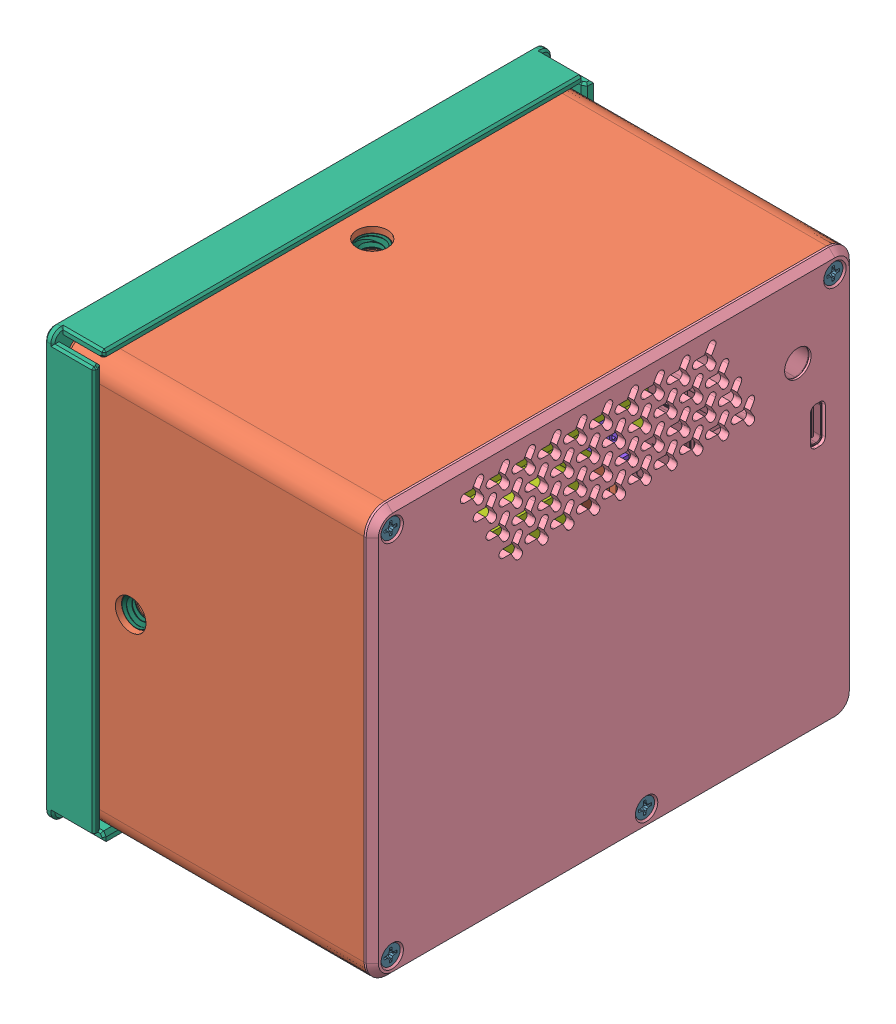
SolidWorks assembly uv_lamp, configuration Default. Lengths in mm.
Overall size (78 104 122.01).
41 component instances, 19 part files, 112 mates.
Components (placement in the parent):
- ushio_care222_emitter-1: ushio_care222_emitter [Default] at (-13.9811 37.7269 -247.0512) size (20.2 75 97)
- housing-1: housing [Default] at (-50.6111 37.7269 -247.0512) x (0 0 1) z (-1 0 0) size (118 100 74)
- ushio_pxz120i2_ballast-2: ushio_pxz120i2_ballast [Default] at (51.5612 17.3221 -21.1407) size (36.3 82.35 88.9) (hidden)
  - ushio_pxz120i2_ballast-1: ushio_pxz120i2_ballast [Default] at (-69.8823 23.5298 -225.9104) size (34.2 82.35 88.9)
  - b5p-vh_jst_vh_connector-1: b5p-vh_jst_vh_connector [Default] at (-72.3723 -13.5702 16.9396) x (0 0 1) z (0 1 0) size (19.74 14.6 8.5)
  - bm02b-srss-tb_jst_sh_connector.step-1: bm02b-srss-tb_jst_sh_connector.step [Default] at (-72.3223 54.1098 46.3896) x (0 -1 0) z (0 0 1) size (4 4.32 3.6)
  - b04b-xask-1_connector-1: b04b-xask-1_connector [Default] at (-72.3723 23.4298 -22.9134) x (0 1 0) z (0 0 -1) size (12.5 12.2 6.4)
- emitter_pxz120i2_ballast_spacer-1: emitter_pxz120i2_ballast_spacer [Default] at (-30.4111 37.7269 -247.0512) x (0 0 -1) z (1 0 0) size (86.9 80.35 9.6) (hidden)
- 99461a939_m3x6mm_self-tapping_screw-1: 99461a939_m3x6mm_self-tapping_screw [99461A939] at (-20.8111 73.9019 -43.6512) x (0 -0.924225 -0.381849) z (1 0 0) size (5.3 5.3 8.28) (hidden)
- 99461a939_m3x6mm_self-tapping_screw-2: 99461a939_m3x6mm_self-tapping_screw [99461A939] at (-20.8111 73.9019 35.2488) x (0 -0.85199 -0.523557) z (1 0 0) size (5.3 5.3 8.28) (hidden)
- 99461a939_m3x6mm_self-tapping_screw-3: 99461a939_m3x6mm_self-tapping_screw [99461A939] at (-20.8111 1.5519 35.2488) x (0 -0.77839 -0.627782) z (1 0 0) size (5.3 5.3 8.28) (hidden)
- 99461a939_m3x6mm_self-tapping_screw-4: 99461a939_m3x6mm_self-tapping_screw [99461A939] at (-20.8111 1.5519 -43.6512) x (0 -0.716484 -0.697604) z (1 0 0) size (5.3 5.3 8.28) (hidden)
- ha40201v4-1000u-a99_fan-1: ha40201v4-1000u-a99_fan [Default] at (221.2389 27.4969 -23.7012) x (0 -1 0) z (-1 0 0) size (22.3 42.67 42.98)
- back_plate-1: back_plate [Default] at (221.0389 10.2269 -23.7012) x (-1 0 0) z (0 1 0) size (44.2 118 100)
- shim-2: shim [Default] at (-20.8111 37.7269 -247.0512) x (0 0 -1) z (1 0 0) size (10.2 2.89 28.2)
- shim-3: shim [Default] at (-20.8111 280.5769 4.7988) x (0 1 0) z (1 0 0) size (10.2 2.89 28.2)
- lens_cap-1: lens_cap [Default] at (-52.6111 37.7269 -247.0512) x (0 0 1) z (-1 0 0) size (122 104 12)
- ushio_pxz120i3_ballast-1: ushio_pxz120i3_ballast [Default] at (-78.3779 173.9684 -27.9154) x (0 1 0) z (1 0 0) size (84.5 86 35.4)
  - ushio_pxz120i3_ballast-1: ushio_pxz120i3_ballast [Default] at (-132.9915 26.2643 55.9668) size (84.5 86 35.4)
  - b05b-xask-1_connector.step-1: b05b-xask-1_connector.step [Default] at (-132.9915 -15.3357 57.5668) x (1 0 0) z (0 -1 0) size (15 12.2 6.4)
  - bm02b-srss-tb_jst_sh_connector.step-1: bm02b-srss-tb_jst_sh_connector.step [Default] at (-101.4915 58.9693 57.6368) x (-1 0 0) z (0 1 0) size (4 4.32 3.6)
  - b5p-vh_jst_vh_connector-1: b5p-vh_jst_vh_connector [Default] at (-170.4415 26.2643 57.5668) x (0 1 0) z (1 0 0) size (19.74 14.6 8.5)
- emitter_pxz120i3_ballast_spacer-1: emitter_pxz120i3_ballast_spacer [Default] at (-30.4111 37.7269 -247.0512) x (0 0 -1) z (1 0 0) size (84.15 78.21 9.6)
- 99461a939_m3x6mm_self-tapping_screw-6: 99461a939_m3x6mm_self-tapping_screw [99461A939] at (-20.8111 0.4769 -22.6512) x (0 -0.536538 0.843876) z (1 0 0) size (5.3 5.3 8.28)
- 99461a939_m3x6mm_self-tapping_screw-8: 99461a939_m3x6mm_self-tapping_screw [99461A939] at (-20.8111 63.4769 -33.1512) x (0 -0.674924 0.737887) z (1 0 0) size (5.3 5.3 8.28)
- 99461a939_m3x6mm_self-tapping_screw-10: 99461a939_m3x6mm_self-tapping_screw [99461A939] at (-20.8111 63.4769 29.8488) x (0 -0.792804 0.609477) z (1 0 0) size (5.3 5.3 8.28)
- lamp_controller_v1.0-1: lamp_controller_v1.0 [Default] at (21.8289 77.7269 -55.6525) x (-1 0 0) z (0 0 1) size (73.56 65 21.25)
- 91698a242_m2.5x6mm_flat_head_screw-1: 91698a242_m2.5x6mm_flat_head_screw [91698A242] at (-29.4211 68.2269 -36.7012) x (0 0 -1) z (1 0 0) size (4.7 4.7 6.16)
- 91698a242_m2.5x6mm_flat_head_screw-2: 91698a242_m2.5x6mm_flat_head_screw [91698A242] at (-29.4211 68.2269 28.2988) x (0 0 -1) z (1 0 0) size (4.7 4.7 6.16)
- 91698a242_m2.5x6mm_flat_head_screw-3: 91698a242_m2.5x6mm_flat_head_screw [91698A242] at (-29.4211 7.2269 -36.7012) x (0 0 -1) z (1 0 0) size (4.7 4.7 6.16)
- 91698a242_m2.5x6mm_flat_head_screw-4: 91698a242_m2.5x6mm_flat_head_screw [91698A242] at (-29.4211 7.2269 28.2988) x (0 0 -1) z (1 0 0) size (4.7 4.7 6.16)
- 47065t905_t-slot_nut-1: 47065t905_t-slot_nut [47065T905] at (-35.6111 83.3393 -4.2012) x (1 0 0) z (0 1 0) size (25.4 11.25 3.49)
- 47065t905_t-slot_nut-2: 47065t905_t-slot_nut [47065T905] at (-35.6111 37.7269 50.4112) x (-1 0 0) z (0 0 1) size (25.4 11.25 3.49)
- 94180a321_m2.5_threaded_insert-1: 94180a321_m2.5_threaded_insert [94180A321] at (17.6739 -7.2731 49.7988) x (0 0 -1) z (1 0 0) size (4.37 4.37 3.6)
- 94180a321_m2.5_threaded_insert-2: 94180a321_m2.5_threaded_insert [94180A321] at (17.6739 82.7269 49.7988) x (0 0.158553 -0.987351) z (1 0 0) size (4.37 4.37 3.6)
- 94180a321_m2.5_threaded_insert-3: 94180a321_m2.5_threaded_insert [94180A321] at (17.6739 82.7269 -58.2012) x (0 0.282984 -0.959125) z (1 0 0) size (4.37 4.37 3.6)
- 94180a321_m2.5_threaded_insert-4: 94180a321_m2.5_threaded_insert [94180A321] at (17.6739 -7.2731 -12.2012) x (0 0.371154 -0.928571) z (1 0 0) size (4.37 4.37 3.6)
- 91698a242_m2.5x6mm_flat_head_screw-6: 91698a242_m2.5x6mm_flat_head_screw [91698A242] at (21.4889 82.8482 49.9202) x (0 0 -1) z (1 0 0) size (4.7 4.7 6.16)
- 91698a242_m2.5x6mm_flat_head_screw-7: 91698a242_m2.5x6mm_flat_head_screw [91698A242] at (21.4889 82.7269 -58.2012) x (0 0 -1) z (1 0 0) size (4.7 4.7 6.16)
- 91698a242_m2.5x6mm_flat_head_screw-8: 91698a242_m2.5x6mm_flat_head_screw [91698A242] at (21.4889 -7.2731 -12.2012) x (0 0 -1) z (1 0 0) size (4.7 4.7 6.16)
- 91698a242_m2.5x6mm_flat_head_screw-9: 91698a242_m2.5x6mm_flat_head_screw [91698A242] at (21.4889 -7.3944 49.9202) x (0 0 -1) z (1 0 0) size (4.7 4.7 6.16)
Mates (geometry in assembly coordinates):
- InPlace1: in place: plane of ushio_care222_emitter-1 through (-50.6111 4.2269 -39.7012) normal (-1 0 0); plane of ? through (-50.6111 0 0) normal (-1 0 0); moOrthogonalPlaneRef_w of ushio_care222_emitter-1 through (-50.6111 4.2269 -39.7012) normal (-1 0 0); plane of ? through (-50.6111 0 0) normal (0 1 0); plane of ushio_care222_emitter-1 through (-50.6111 4.2269 -39.7012) normal (-1 0 0); plane of ? through (-50.6111 0 0) normal (0 0 1); plane of ushio_care222_emitter-1 through (-50.6111 4.2269 -39.7012) normal (-1 0 0); unknown of housing-1
- Coincident1: coincident aligned: plane of ushio_care222_emitter-1; plane of housing-1
- Coincident2: coincident aligned: moOrthogonalPlaneRef_w of ushio_care222_emitter-1 through (-50.6111 37.7269 -247.0512) normal (0 1 0); plane of housing-1 through (-50.6111 37.7269 -247.0512) normal (0 1 0)
- Coincident3: coincident anti-aligned: moOrthogonalPlaneRef_w of ushio_care222_emitter-1 through (-50.6111 37.7269 -247.0512) normal (0 0 -1); plane of housing-1 through (-50.6111 37.7269 -247.0512) normal (0 0 1)
- Parallel1: parallel anti-aligned: plane of ushio_care222_emitter-1 through (-30.4111 4.2269 31.2988) normal (1 0 0); plane of ushio_pxz120i2_ballast-2/ushio_pxz120i2_ballast-1 through (-22.4111 40.8519 -247.0512) normal (-1 0 0)
- Parallel2: parallel aligned: plane of ushio_care222_emitter-1 through (-50.6111 0.2269 31.2988) normal (0 -1 0); plane of ushio_pxz120i2_ballast-2/ushio_pxz120i2_ballast-1 through (-22.4111 -3.4481 -247.0512) normal (0 -1 0)
- Width1: width anti-aligned: plane of ushio_pxz120i2_ballast-2/ushio_pxz120i2_ballast-1 through (-22.4111 -3.4481 -247.0512) normal (0 -1 0); plane of ushio_care222_emitter-1 through (-22.4111 78.9019 -247.0512) normal (0 1 0); plane of ushio_pxz120i2_ballast-2/ushio_pxz120i2_ballast-1 through (-50.6111 75.2269 31.2988) normal (0 1 0); plane of ushio_care222_emitter-1 through (-50.6111 0.2269 31.2988) normal (0 -1 0)
- Width2: width anti-aligned: plane of ushio_pxz120i2_ballast-2/ushio_pxz120i2_ballast-1 through (-22.4111 40.8519 40.2488) normal (0 0 1); plane of ushio_care222_emitter-1 through (-22.4111 40.8519 -48.6512) normal (0 0 -1); plane of ushio_pxz120i2_ballast-2/ushio_pxz120i2_ballast-1 through (-50.6111 4.2269 -43.7012) normal (0 0 -1); plane of ushio_care222_emitter-1 through (-50.6111 4.2269 35.2988) normal (0 0 1)
- Distance1: distance anti-aligned: plane of ushio_care222_emitter-1 through (-30.4111 4.2269 31.2988) normal (1 0 0); plane of ushio_pxz120i2_ballast-2/ushio_pxz120i2_ballast-1 through (-22.4111 40.8519 -247.0512) normal (-1 0 0)
- InPlace2: in place: plane of ushio_care222_emitter-1 through (-30.4111 4.2269 31.2988) normal (1 0 0); plane of ? through (-30.4111 0 0) normal (1 0 0); plane of ushio_care222_emitter-1 through (-30.4111 4.2269 31.2988) normal (1 0 0); plane of ? through (-30.4111 0 0) normal (0 1 0); plane of ushio_care222_emitter-1 through (-30.4111 4.2269 31.2988) normal (1 0 0); plane of ? through (-30.4111 0 0) normal (0 0 -1); plane of ushio_care222_emitter-1 through (-30.4111 4.2269 31.2988) normal (1 0 0); unknown of ?
- Coincident1: coincident aligned: plane of ushio_care222_emitter-1; plane of emitter_pxz120i2_ballast_spacer-1
- Coincident2: coincident aligned: moOrthogonalPlaneRef_w of ushio_care222_emitter-1 through (-30.4111 37.7269 -247.0512) normal (0 1 0); plane of emitter_pxz120i2_ballast_spacer-1 through (-30.4111 37.7269 -247.0512) normal (0 1 0)
- Coincident3: coincident anti-aligned: moOrthogonalPlaneRef_w of ushio_care222_emitter-1 through (-30.4111 37.7269 -247.0512) normal (0 0 1); plane of emitter_pxz120i2_ballast_spacer-1 through (-30.4111 37.7269 -247.0512) normal (0 0 -1)
- Distance19: distance = 0.5 mm anti-aligned: plane of housing-1 through (21.3889 -10.2731 -247.0512) normal (0 1 0); plane of ha40201v4-1000u-a99_fan-1 through (1.3889 -9.7731 -39.2012) normal (0 -1 0)
- Distance13: distance anti-aligned: plane of housing-1 through (21.3889 37.7269 -61.2012) normal (0 0 1); plane of ha40201v4-1000u-a99_fan-1 through (21.3889 -9.7731 -59.2012) normal (0 0 -1)
- Parallel8: parallel aligned: plane of ushio_care222_emitter-1 through (-50.6111 4.2269 -39.7012) normal (-1 0 0); plane of hlk-ld2410c_radar-1 through (-49.0111 37.7269 -52.2012) normal (-1 0 0)
- Distance12: distance anti-aligned: plane of ushio_care222_emitter-1 through (-50.6111 4.2269 -43.7012) normal (0 0 -1); plane of hlk-ld2410c_radar-1 through (-47.4111 26.6769 -44.2012) normal (0 0 1)
- Coincident18: coincident aligned: plane of ushio_care222_emitter-1 through (-50.6111 4.2269 -39.7012) normal (-1 0 0); plane of hlk-ld2410c_radar-1 through (-50.6111 37.7269 -52.2012) normal (-1 0 0)
- Coincident20: coincident anti-aligned: plane of housing-1 through (-50.6111 37.7269 -247.0512) normal (0 1 0); plane of hlk-ld2410c_radar-1 through (-49.0111 37.7269 -52.2012) normal (0 -1 0)
- Coincident30: coincident anti-aligned: plane of back_plate-1 through (21.3889 -7.2731 49.7988) normal (-1 0 0); plane of housing-1 through (21.3889 37.7269 -247.0512) normal (1 0 0)
- Distance14: distance = 1.5 mm anti-aligned: plane of ushio_pxz120i2_ballast-2/ushio_pxz120i2_ballast-1 through (9.1889 60.1019 -27.7012) normal (0 -1 0); plane of rp2040_controller_v1.0-1 through (10.5762 58.6019 -40.6512) normal (0 1 0)
- Distance18: distance = 5 mm: plane of rp2040_controller_v1.0-1 through (10.5762 15.6019 -43.6512) normal (0 0 -1); line of ushio_pxz120i2_ballast-2/ushio_pxz120i2_ballast-1 through (-20.8111 76.9019 -48.6512) axis (0 -1 0)
- Concentric1: concentric anti-aligned: cylinder of housing-1 through (-35.6111 64.5953 -4.2012) axis (0 -1 0) radius 3.75; cylinder of 47065t905_t-slot_nut-1 through (-35.6111 83.1818 -4.2012) axis (0 1 0) radius 3.5687
- Parallel10: parallel anti-aligned: plane of housing-1 through (-50.6111 37.7269 -9.8012) normal (0 0 1); plane of 47065t905_t-slot_nut-1 through (-25.0601 83.3393 -9.8273) normal (0 0 -1)
- Coincident33: coincident anti-aligned: plane of housing-1 through (21.3889 85.7269 -247.0512) normal (0 -1 0); plane of 47065t905_t-slot_nut-1 through (-35.6111 85.7269 -4.2012) normal (0 1 0)
- Concentric2: concentric aligned: cylinder of housing-1 through (-35.6111 37.7269 54.7988) axis (0 0 1) radius 3.75; cylinder of 47065t905_t-slot_nut-2 through (-35.6111 37.7269 50.2538) axis (0 0 1) radius 3.5687
- Parallel11: parallel anti-aligned: plane of housing-1 through (-50.6111 32.1269 -247.0512) normal (0 1 0); plane of 47065t905_t-slot_nut-2 through (-46.1621 32.1008 50.4112) normal (0 -1 0)
- Coincident34: coincident anti-aligned: plane of housing-1 through (21.3889 37.7269 52.7988) normal (0 0 -1); plane of 47065t905_t-slot_nut-2 through (-35.6111 37.7269 52.7988) normal (0 0 1)
- InPlace4: in place: plane of housing-1 through (-50.6111 43.2269 47.3988) normal (0 0 -1); plane of ? through (0 0 47.3988) normal (0 0 -1); plane of housing-1 through (-50.6111 43.2269 47.3988) normal (0 0 -1); plane of ? through (0 0 47.3988) normal (0 1 0); plane of housing-1 through (-50.6111 43.2269 47.3988) normal (0 0 -1); plane of ? through (0 0 47.3988) normal (-1 0 0); plane of housing-1 through (-50.6111 42.9769 47.3988) normal (0 0 -1); unknown of ?
- Coincident35: coincident aligned: plane of housing-1; plane of ?
- Coincident36: coincident aligned: moOrthogonalPlaneRef_w of housing-1 through (-50.6111 37.7269 47.3988) normal (0 1 0); plane of shim1-1 through (-50.6111 37.7269 47.3988) normal (0 1 0)
- Coincident37: coincident anti-aligned: moOrthogonalPlaneRef_w of housing-1 through (-50.6111 37.7269 47.3988) normal (1 0 0); plane of shim1-1 through (-50.6111 37.7269 47.3988) normal (-1 0 0)
- InPlace5: in place: plane of housing-1 through (-22.4111 40.8519 -247.0512) normal (1 0 0); plane of ? through (-22.4111 0 0) normal (1 0 0); plane of housing-1 through (-22.4111 40.8519 -247.0512) normal (1 0 0); plane of ? through (-22.4111 0 0) normal (0 1 0); plane of housing-1 through (-22.4111 40.8519 -247.0512) normal (1 0 0); plane of ? through (-22.4111 0 0) normal (0 0 -1); plane of housing-1 through (-22.4111 40.8519 -247.0512) normal (1 0 0); unknown of ?
- Coincident38: coincident aligned: plane of housing-1; plane of ?
- Coincident39: coincident aligned: moOrthogonalPlaneRef_w of housing-1 through (-22.4111 37.7269 -247.0512) normal (0 1 0); plane of shim2-1 through (-22.4111 37.7269 -247.0512) normal (0 1 0)
- Coincident40: coincident anti-aligned: moOrthogonalPlaneRef_w of housing-1 through (-22.4111 37.7269 -247.0512) normal (0 0 1); plane of shim2-1 through (-22.4111 37.7269 -247.0512) normal (0 0 -1)
- InPlace6: in place: plane of housing-1 through (-20.8111 43.2269 -247.0512) normal (1 0 0); plane of ? through (-20.8111 0 0) normal (1 0 0); plane of housing-1 through (-20.8111 43.2269 -247.0512) normal (1 0 0); plane of ? through (-20.8111 0 0) normal (0 1 0); plane of housing-1 through (-20.8111 43.2269 -247.0512) normal (1 0 0); plane of ? through (-20.8111 0 0) normal (0 0 -1); plane of housing-1 through (-20.8111 42.9769 -247.0512) normal (1 0 0); unknown of shim-2
- Coincident35: coincident aligned: plane of housing-1; plane of shim-2
- Coincident36: coincident aligned: moOrthogonalPlaneRef_w of housing-1 through (-20.8111 37.7269 -247.0512) normal (0 1 0); plane of shim-2 through (-20.8111 37.7269 -247.0512) normal (0 1 0)
- Coincident37: coincident anti-aligned: moOrthogonalPlaneRef_w of housing-1 through (-20.8111 37.7269 -247.0512) normal (0 0 1); plane of shim-2 through (-20.8111 37.7269 -247.0512) normal (0 0 -1)
- InPlace7: in place: plane of housing-1 through (-52.6111 37.7269 -247.0512) normal (-1 0 0); plane of ? through (-52.6111 0 0) normal (-1 0 0); plane of housing-1 through (-52.6111 37.7269 -247.0512) normal (-1 0 0); plane of ? through (-52.6111 0 0) normal (0 1 0); plane of housing-1 through (-52.6111 37.7269 -247.0512) normal (-1 0 0); plane of ? through (-52.6111 0 0) normal (0 0 1); plane of housing-1 through (-52.6111 37.7269 -247.0512) normal (-1 0 0); unknown of lens_cap-1
- Coincident35: coincident aligned: plane of housing-1; plane of lens_cap-1
- Coincident36: coincident aligned: moOrthogonalPlaneRef_w of housing-1 through (-52.6111 37.7269 -247.0512) normal (0 1 0); plane of lens_cap-1 through (-52.6111 37.7269 -247.0512) normal (0 1 0)
- Coincident37: coincident anti-aligned: moOrthogonalPlaneRef_w of housing-1 through (-52.6111 37.7269 -247.0512) normal (0 0 -1); plane of lens_cap-1 through (-52.6111 37.7269 -247.0512) normal (0 0 1)
- Parallel12: parallel aligned: plane of ushio_care222_emitter-1 through (-50.6111 75.2269 31.2988) normal (0 1 0); plane of ushio_pxz120i3_ballast-1/ushio_pxz120i3_ballast-1 through (-20.8111 79.9769 35.9346) normal (0 1 0)
- Parallel13: parallel aligned: plane of ushio_care222_emitter-1 through (-50.6111 4.2269 -43.7012) normal (0 0 -1); plane of ushio_pxz120i3_ballast-1/ushio_pxz120i3_ballast-1 through (-20.8111 52.5627 -48.6512) normal (0 0 -1)
- Distance20: distance anti-aligned: plane of ushio_pxz120i3_ballast-1/ushio_pxz120i3_ballast-1 through (-22.4111 40.9769 -1.6512) normal (-1 0 0); plane of ushio_care222_emitter-1 through (-30.4111 4.2269 31.2988) normal (1 0 0)
- Width3: width anti-aligned: plane of ushio_pxz120i3_ballast-1/ushio_pxz120i3_ballast-1 through (-20.8111 79.9769 -18.1512) normal (0 1 0); plane of ushio_care222_emitter-1 through (-20.8111 -4.5231 -27.6512) normal (0 -1 0); plane of ushio_pxz120i3_ballast-1/ushio_pxz120i3_ballast-1 through (-50.6111 0.2269 31.2988) normal (0 -1 0); plane of ushio_care222_emitter-1 through (-50.6111 75.2269 31.2988) normal (0 1 0)
- Coincident35: coincident aligned: plane of ushio_pxz120i2_ballast-2/ushio_pxz120i2_ballast-1 through (-22.4111 40.8519 -48.6512) normal (0 0 -1); plane of ushio_pxz120i3_ballast-1/ushio_pxz120i3_ballast-1 through (-20.8111 52.5627 -48.6512) normal (0 0 -1)
- Distance21: distance = 4 mm: plane of lamp_controller_v1.0_3d_model.step-1 through (-10.6713 45.6771 -57.2012) normal (0 0 -1); plane of housing-1 through (21.3889 37.7269 -61.2012) normal (0 0 1)
- Coincident37: coincident: plane of housing-1 through (-49.0111 37.7269 -247.0512) normal (1 0 0); line of lamp_controller_v1.0_3d_model.step-1 through (-49.0111 28.6269 -43.9639) axis (0 1 0)
- Coincident38: coincident: plane of housing-1 through (-30.6111 49.2269 -247.0512) normal (0 -1 0); line of lamp_controller_v1.0_3d_model.step-1 through (-49.0111 49.2269 -45.4639) axis (1 0 0)
- Distance22: distance = 4 mm anti-aligned: plane of lamp_controller_v1.0-1 through (-13.0343 46.4966 -57.2012) normal (0 0 -1); plane of housing-1 through (21.3889 37.7269 -61.2012) normal (0 0 1)
- Symmetric2: symmetric aligned: plane of housing-1 through (-30.6111 26.2269 -247.0512) normal (0 1 0); plane of lamp_controller_v1.0-1 through (-30.6111 49.2269 -247.0512) normal (0 -1 0); plane of housing-1 through (21.8289 37.7269 -55.6525) normal (0 -1 0)
- Coincident41: coincident anti-aligned: plane of housing-1 through (-49.0111 37.7269 -247.0512) normal (1 0 0); plane of lamp_controller_v1.0-1 through (-49.0111 77.7269 -55.6525) normal (-1 0 0)
- Concentric3: concentric aligned: cylinder of ushio_pxz120i2_ballast-2/ushio_pxz120i2_ballast-1 through (-22.4111 73.9019 -43.6512) axis (1 0 0) radius 1.75; cylinder of 99461a939_m3x6mm_self-tapping_screw-1 through (-18.7111 73.9019 -43.6512) axis (1 0 0) radius 2.65
- Coincident42: coincident anti-aligned: plane of ushio_pxz120i2_ballast-2/ushio_pxz120i2_ballast-1 through (-20.8111 40.8519 -4.2012) normal (1 0 0); plane of 99461a939_m3x6mm_self-tapping_screw-1 through (-20.8111 74.2188 -44.4183) normal (-1 0 0)
- Coincident43: coincident anti-aligned: plane of ushio_pxz120i2_ballast-2/ushio_pxz120i2_ballast-1 through (-20.8111 40.8519 -4.2012) normal (1 0 0); plane of 99461a939_m3x6mm_self-tapping_screw-2 through (-20.8111 74.3365 34.5417) normal (-1 0 0)
- Concentric4: concentric aligned: cylinder of ushio_pxz120i2_ballast-2/ushio_pxz120i2_ballast-1 through (-22.4111 73.9019 35.2488) axis (1 0 0) radius 1.75; cylinder of 99461a939_m3x6mm_self-tapping_screw-2 through (-18.7111 73.9019 35.2488) axis (1 0 0) radius 2.65
- Coincident44: coincident anti-aligned: plane of ushio_pxz120i2_ballast-2/ushio_pxz120i2_ballast-1 through (-20.8111 40.8519 -4.2012) normal (1 0 0); plane of 99461a939_m3x6mm_self-tapping_screw-3 through (-20.8111 2.073 34.6028) normal (-1 0 0)
- Concentric5: concentric aligned: cylinder of ushio_pxz120i2_ballast-2/ushio_pxz120i2_ballast-1 through (-22.4111 1.5519 35.2488) axis (1 0 0) radius 1.75; cylinder of 99461a939_m3x6mm_self-tapping_screw-3 through (-18.7111 1.5519 35.2488) axis (1 0 0) radius 2.65
- Coincident45: coincident anti-aligned: plane of ushio_pxz120i2_ballast-2/ushio_pxz120i2_ballast-1 through (-20.8111 40.8519 -4.2012) normal (1 0 0); plane of 99461a939_m3x6mm_self-tapping_screw-4 through (-20.8111 2.1309 -44.2458) normal (-1 0 0)
- Concentric6: concentric aligned: cylinder of ushio_pxz120i2_ballast-2/ushio_pxz120i2_ballast-1 through (-22.4111 1.5519 -43.6512) axis (1 0 0) radius 1.75; cylinder of 99461a939_m3x6mm_self-tapping_screw-4 through (-18.7111 1.5519 -43.6512) axis (1 0 0) radius 2.65
- Coincident47: coincident aligned: cone of emitter_pxz120i2_ballast_spacer-1 through (-27.4111 68.2269 -36.7012) axis (-1 0 0); cone of 91698a242_m2.5x6mm_flat_head_screw-1 through (-27.9211 68.2269 -36.7012) axis (-1 0 0)
- Parallel14: parallel aligned: plane of 91698a242_m2.5x6mm_flat_head_screw-1 through (-29.4211 68.2269 -36.7012) normal (0 1 0)
- Parallel15: parallel aligned: plane of 91698a242_m2.5x6mm_flat_head_screw-2 through (-29.4211 68.2269 28.2988) normal (0 1 0)
- Coincident49: coincident aligned: cone of emitter_pxz120i2_ballast_spacer-1 through (-27.4111 68.2269 28.2988) axis (-1 0 0); cone of 91698a242_m2.5x6mm_flat_head_screw-2 through (-27.9211 68.2269 28.2988) axis (-1 0 0)
- Parallel16: parallel aligned: plane of 91698a242_m2.5x6mm_flat_head_screw-3 through (-29.4211 7.2269 -36.7012) normal (0 1 0)
- Coincident50: coincident aligned: cone of emitter_pxz120i2_ballast_spacer-1 through (-27.4111 7.2269 -36.7012) axis (-1 0 0); cone of 91698a242_m2.5x6mm_flat_head_screw-3 through (-27.9211 7.2269 -36.7012) axis (-1 0 0)
- Parallel17: parallel aligned: plane of 91698a242_m2.5x6mm_flat_head_screw-4 through (-29.4211 7.2269 28.2988) normal (0 1 0)
- Coincident51: coincident aligned: cone of emitter_pxz120i2_ballast_spacer-1 through (-27.4111 7.2269 28.2988) axis (-1 0 0); cone of 91698a242_m2.5x6mm_flat_head_screw-4 through (-27.9211 7.2269 28.2988) axis (-1 0 0)
- Concentric7: concentric anti-aligned: cylinder of ushio_pxz120i3_ballast-1/ushio_pxz120i3_ballast-1 through (-20.8111 0.4769 -22.6512) axis (-1 0 0) radius 1.6; cylinder of 99461a939_m3x6mm_self-tapping_screw-6 through (-18.7111 0.4769 -22.6512) axis (1 0 0) radius 2.65
- Coincident52: coincident anti-aligned: plane of ushio_pxz120i3_ballast-1/ushio_pxz120i3_ballast-1 through (-20.8111 40.9769 -1.6512) normal (1 0 0); plane of 99461a939_m3x6mm_self-tapping_screw-6 through (-20.8111 -0.2235 -23.0965) normal (-1 0 0)
- Concentric8: concentric anti-aligned: cylinder of ushio_pxz120i3_ballast-1/ushio_pxz120i3_ballast-1 through (-20.8111 63.4769 -33.1512) axis (-1 0 0) radius 1.6; cylinder of 99461a939_m3x6mm_self-tapping_screw-8 through (-18.7111 63.4769 -33.1512) axis (1 0 0) radius 2.65
- Coincident54: coincident anti-aligned: plane of ushio_pxz120i3_ballast-1/ushio_pxz120i3_ballast-1 through (-20.8111 40.9769 -1.6512) normal (1 0 0); plane of 99461a939_m3x6mm_self-tapping_screw-8 through (-20.8111 62.8645 -33.7113) normal (-1 0 0)
- Concentric9: concentric anti-aligned: cylinder of ushio_pxz120i3_ballast-1/ushio_pxz120i3_ballast-1 through (-20.8111 63.4769 29.8488) axis (-1 0 0) radius 1.6; cylinder of 99461a939_m3x6mm_self-tapping_screw-10 through (-18.7111 63.4769 29.8488) axis (1 0 0) radius 2.65
- Coincident55: coincident anti-aligned: plane of ushio_pxz120i3_ballast-1/ushio_pxz120i3_ballast-1 through (-20.8111 40.9769 -1.6512) normal (1 0 0); plane of 99461a939_m3x6mm_self-tapping_screw-10 through (-20.8111 62.971 29.1908) normal (-1 0 0)
- Concentric10: concentric aligned: cylinder of housing-1 through (14.3889 -7.2731 49.7988) axis (1 0 0) radius 1.93; cylinder of 94180a321_m2.5_threaded_insert-1 through (19.3889 -7.2731 49.7988) axis (1 0 0) radius 1.8089
- Coincident56: coincident aligned: plane of housing-1 through (19.3889 37.7269 -247.0512) normal (1 0 0); plane of 94180a321_m2.5_threaded_insert-1 through (19.3889 -6.0231 49.7988) normal (1 0 0)
- Coincident57: coincident aligned: plane of housing-1 through (19.3889 37.7269 -247.0512) normal (1 0 0); plane of 94180a321_m2.5_threaded_insert-2 through (19.3889 83.9611 49.997) normal (1 0 0)
- Concentric11: concentric aligned: cylinder of housing-1 through (14.3889 82.7269 49.7988) axis (1 0 0) radius 1.93; cylinder of 94180a321_m2.5_threaded_insert-2 through (19.3889 82.7269 49.7988) axis (1 0 0) radius 1.8089
- Coincident58: coincident aligned: plane of housing-1 through (19.3889 37.7269 -247.0512) normal (1 0 0); plane of 94180a321_m2.5_threaded_insert-3 through (19.3889 83.9258 -57.8474) normal (1 0 0)
- Concentric12: concentric aligned: cylinder of housing-1 through (14.3889 82.7269 -58.2012) axis (1 0 0) radius 1.93; cylinder of 94180a321_m2.5_threaded_insert-3 through (19.3889 82.7269 -58.2012) axis (1 0 0) radius 1.8089
- Coincident59: coincident aligned: plane of housing-1 through (19.3889 37.7269 -247.0512) normal (1 0 0); plane of 94180a321_m2.5_threaded_insert-4 through (19.3889 -6.1124 -11.7372) normal (1 0 0)
- Concentric13: concentric aligned: cylinder of housing-1 through (14.3889 -7.2731 -12.2012) axis (1 0 0) radius 1.93; cylinder of 94180a321_m2.5_threaded_insert-4 through (19.3889 -7.2731 -12.2012) axis (1 0 0) radius 1.8089
- Coincident61: coincident aligned: cone of back_plate-1 through (23.3889 82.8482 49.9202) axis (-1 0 0); cone of 91698a242_m2.5x6mm_flat_head_screw-6 through (22.9889 82.8482 49.9202) axis (-1 0 0)
- Parallel20: parallel aligned: plane of 91698a242_m2.5x6mm_flat_head_screw-7 through (21.4889 82.7269 -58.2012) normal (0 1 0)
- Coincident62: coincident aligned: cone of back_plate-1 through (23.3889 82.7269 -58.2012) axis (-1 0 0); cone of 91698a242_m2.5x6mm_flat_head_screw-7 through (22.9889 82.7269 -58.2012) axis (-1 0 0)
- Parallel21: parallel aligned: plane of 91698a242_m2.5x6mm_flat_head_screw-8 through (21.4889 -7.2731 -12.2012) normal (0 1 0)
- Coincident63: coincident aligned: cone of back_plate-1 through (23.3889 -7.2731 -12.2012) axis (-1 0 0); cone of 91698a242_m2.5x6mm_flat_head_screw-8 through (22.9889 -7.2731 -12.2012) axis (-1 0 0)
- Parallel22: parallel aligned: plane of 91698a242_m2.5x6mm_flat_head_screw-9 through (21.4889 -7.3944 49.9202) normal (0 1 0)
- Coincident64: coincident aligned: cone of back_plate-1 through (23.3889 -7.3944 49.9202) axis (-1 0 0); cone of 91698a242_m2.5x6mm_flat_head_screw-9 through (22.9889 -7.3944 49.9202) axis (-1 0 0)
- Width4: width anti-aligned: plane of diffuser_hoop-1/diffuser_outer_hoop-1 through (-55.6111 87.7269 -32.7512) normal (0 1 0); plane of housing-1 through (-55.6111 -12.2731 -32.7512) normal (0 -1 0); plane of diffuser_hoop-1/diffuser_outer_hoop-1 through (-52.6111 -12.2731 -247.0512) normal (0 -1 0); plane of housing-1 through (-52.6111 87.7269 -247.0512) normal (0 1 0)
- Width5: width aligned: plane of diffuser_hoop-1/diffuser_outer_hoop-1 through (-55.6111 3.7269 40.3488) normal (0 0 1); plane of housing-1 through (-55.6111 3.7269 -48.7512) normal (0 0 -1); plane of diffuser_hoop-1/diffuser_outer_hoop-1 through (-52.6111 37.7269 54.7988) normal (0 0 1); plane of housing-1 through (-52.6111 37.7269 -63.2012) normal (0 0 -1)
- Coincident67: coincident anti-aligned: plane of housing-1 through (-52.6111 37.7269 -247.0512) normal (-1 0 0); plane of diffuser_hoop-1/magnet-2 through (-52.6111 -9.2731 15.7988) normal (1 0 0)
- Coincident69: coincident anti-aligned: plane of housing-1 through (-30.6111 37.7269 44.7988) normal (0 0 1); plane of shim-3 through (-30.8111 280.5769 44.7988) normal (0 0 -1)
- Width6: width anti-aligned: plane of shim-3 through (-30.8111 42.8269 7.9238) normal (0 1 0); plane of shim-3 through (-30.8111 32.6269 7.9238) normal (0 -1 0); plane of housing-1 through (-50.6111 43.3269 -247.0512) normal (0 -1 0); plane of housing-1 through (-50.6111 32.1269 -247.0512) normal (0 1 0)
- Coincident71: coincident anti-aligned: plane of housing-1 through (-50.6111 37.7269 -247.0512) normal (1 0 0); plane of shim-3 through (-50.6111 32.1269 52.7988) normal (-1 0 0)
- Concentric14: concentric aligned: cylinder of housing-1 through (-35.6111 37.7269 54.7988) axis (0 0 1) radius 3.75; cylinder of goniometer_bracket-1 through (-35.6111 37.7269 -66.2022) axis (0 0 1) radius 3.2639
- Concentric15: concentric aligned: cylinder of housing-1 through (-35.6111 64.5953 -4.2012) axis (0 1 0) radius 3.75; cylinder of goniometer_bracket-1 through (-35.6111 -15.2741 -4.2012) axis (0 1 0) radius 3.2639
- InPlace8: in place: plane of housing-1 through (-52.6111 37.7269 -247.0512) normal (-1 0 0); plane of ? through (-52.6111 0 0) normal (-1 0 0); plane of housing-1 through (-52.6111 37.7269 -247.0512) normal (-1 0 0); plane of ? through (-52.6111 0 0) normal (0 1 0); plane of housing-1 through (-52.6111 37.7269 -247.0512) normal (-1 0 0); plane of ? through (-52.6111 0 0) normal (0 0 1); plane of housing-1 through (-52.6111 37.7269 -247.0512) normal (-1 0 0); unknown of lens_cap-1
- Coincident73: coincident aligned: plane of housing-1; plane of ?
- Coincident74: coincident aligned: moOrthogonalPlaneRef_w of housing-1 through (-52.6111 37.7269 -247.0512) normal (0 1 0); plane of corrugated_diffuser_clamp_1-1 through (-52.6111 37.7269 -247.0512) normal (0 1 0)
- Coincident75: coincident anti-aligned: moOrthogonalPlaneRef_w of housing-1 through (-52.6111 37.7269 -247.0512) normal (0 0 -1); plane of corrugated_diffuser_clamp_1-1 through (-52.6111 37.7269 -247.0512) normal (0 0 1)
- Concentric16: concentric aligned: cylinder of housing-1 through (-35.6111 64.5953 -4.2012) axis (0 1 0) radius 3.75; cylinder of straight_diffuser_clamp_1-1 through (-35.6111 -22.2741 -4.2012) axis (0 1 0) radius 3.2639
- Concentric17: concentric aligned: cylinder of goniometer_bracket-1 through (-35.6111 37.7269 -66.2022) axis (0 0 1) radius 3.2639; cylinder of straight_diffuser_clamp_1-1 through (-35.6111 37.7269 -66.2022) axis (0 0 1) radius 3.2639
- Coincident72: coincident aligned: plane of housing-1 through (-52.6111 -12.2731 -247.0512) normal (0 -1 0); plane of back_plate-1 through (23.3889 -12.2731 49.7988) normal (0 -1 0)
- Coincident73: coincident aligned: plane of housing-1 through (-52.6111 37.7269 -63.2012) normal (0 0 -1); plane of back_plate-1 through (23.3889 -7.2731 -63.2012) normal (0 0 -1)
- Parallel23: parallel aligned: plane of back_plate-1 through (23.3889 87.7269 49.7988) normal (0 1 0); plane of 91698a242_m2.5x6mm_flat_head_screw-6 through (21.4889 82.8482 49.9202) normal (0 1 0)
- Coincident74: coincident anti-aligned: plane of ha40201v4-1000u-a99_fan-1 through (21.3889 -9.7731 -19.2012) normal (1 0 0); plane of back_plate-1 through (21.3889 -7.2731 49.7988) normal (-1 0 0)
- Concentric19: concentric aligned: cylinder of straight_diffuser_clamp_1-1 through (-55.6111 68.2269 -57.7012) axis (1 0 0) radius 3; cylinder of cylinder_magnet-1 through (-55.1111 68.2269 -57.7012) axis (1 0 0) radius 3
- Coincident76: coincident aligned: plane of straight_diffuser_clamp_1-1 through (-52.6111 37.7269 -247.0512) normal (1 0 0); plane of cylinder_magnet-1 through (-52.6111 68.2269 -57.7012) normal (1 0 0)
